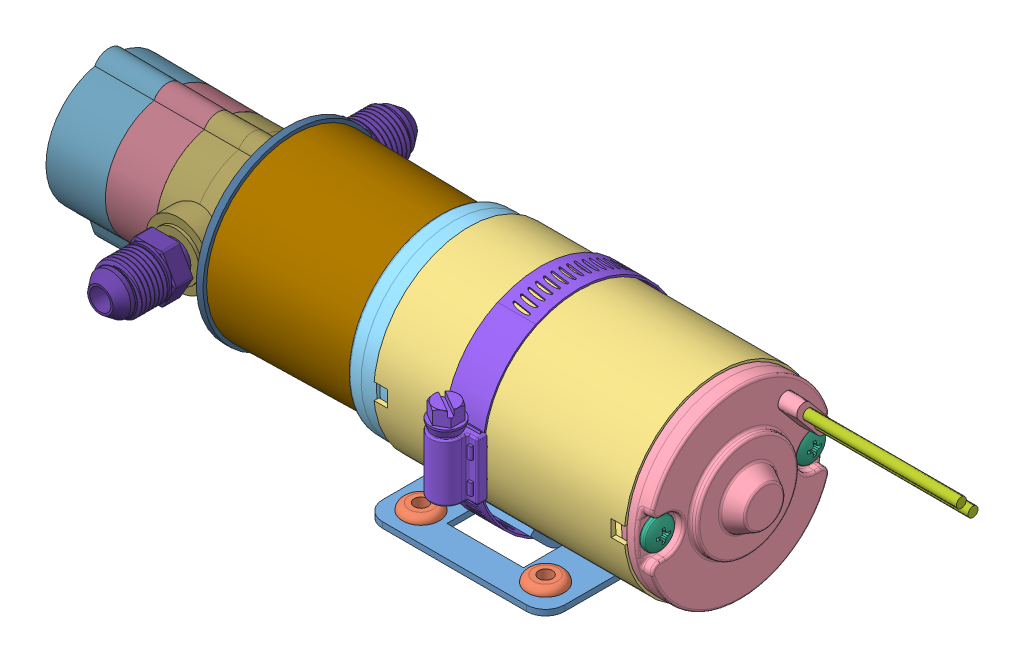
SolidWorks assembly P-SERIES, configuration Default. Lengths in mm.
Overall size (266.07 68.69 100.84).
26 component instances, 17 part files, 51 mates.
Components (placement in the parent):
- BAND CLAMP MOUNTING PLATE^P-SERIES-1: BAND CLAMP MOUNTING PLATE^P-SERIES [Default] at origin size (60.32 13.25 69.85) (virtual)
  - BAND CLAMP MOUNTING PLATE^BAND CLAMP MOUNTING PLATE_P-SERIES-1: BAND CLAMP MOUNTING PLATE^BAND CLAMP MOUNTING PLATE_P-SERIES [01] at (0 1.905 0) x (0 0 1) z (0 -1 0) size (69.85 60.32 11.06) (virtual)
  - GROMMET^BAND CLAMP MOUNTING PLATE_P-SERIES-1: GROMMET^BAND CLAMP MOUNTING PLATE_P-SERIES [01] at (20.6375 1.016 -25.4) size (12.19 6.4 12.19) (virtual)
  - GROMMET^BAND CLAMP MOUNTING PLATE_P-SERIES-2: GROMMET^BAND CLAMP MOUNTING PLATE_P-SERIES [01] at (-20.6375 1.016 -25.4) size (12.19 6.4 12.19) (virtual)
  - GROMMET^BAND CLAMP MOUNTING PLATE_P-SERIES-3: GROMMET^BAND CLAMP MOUNTING PLATE_P-SERIES [01] at (20.6375 1.016 25.4) size (12.19 6.4 12.19) (virtual)
  - GROMMET^BAND CLAMP MOUNTING PLATE_P-SERIES-4: GROMMET^BAND CLAMP MOUNTING PLATE_P-SERIES [01] at (-20.6375 1.016 25.4) size (12.19 6.4 12.19) (virtual)
- 12VDC MOTOR^P-SERIES-1: 12VDC MOTOR^P-SERIES [Default] at (11.3375 34.421 0) size (156.2 63 63) (virtual)
  - 12VDC MOTOR HOUSING^12VDC MOTOR_P-SERIES-1: 12VDC MOTOR HOUSING^12VDC MOTOR_P-SERIES [01] at origin size (83 63 63) (virtual)
  - SOURCE END CASTING^12VDC MOTOR_P-SERIES-1: SOURCE END CASTING^12VDC MOTOR_P-SERIES [01] at origin size (18.93 61.6 61.6) (virtual)
  - COUPLER END CASTING^12VDC MOTOR_P-SERIES-1: COUPLER END CASTING^12VDC MOTOR_P-SERIES [01] at origin size (12.31 61.6 61.6) (virtual)
  - PHIL MACHINE SCREW^12VDC MOTOR_P-SERIES-1: PHIL MACHINE SCREW^12VDC MOTOR_P-SERIES [93802A733] at (28.998 0 25) x (0 1 0) z (1 0 0) size (10.35 10.24 95.59) (virtual)
  - PHIL MACHINE SCREW^12VDC MOTOR_P-SERIES-2: PHIL MACHINE SCREW^12VDC MOTOR_P-SERIES [93802A733] at (28.998 0 -25) x (0 1 0) z (1 0 0) size (10.35 10.24 95.59) (virtual)
  - WIRES^12VDC MOTOR_P-SERIES-1: WIRES^12VDC MOTOR_P-SERIES [01] at (54.5 0 0) x (0 0 -1) z (1 0 0) size (7.16 7.9 57.15) (virtual)
- WORM-DRIVE CLAMP^P-SERIES-1: WORM-DRIVE CLAMP^P-SERIES [01] at (0 32.5835 0) x (0 1 0) z (1 0 0) size (67.85 76.82 17.02) (virtual)
- COUPLER^P-SERIES-1: COUPLER^P-SERIES [01] at (-63.8125 34.421 0) size (48.5 58 58) (virtual)
- COUPLER PLATE^P-SERIES-1: COUPLER PLATE^P-SERIES [01] at (-88.0625 34.421 0) x (0 0 1) z (-1 0 0) size (60.3 60.3 2.25) (virtual)
- Socket Head Screw^P-SERIES-1: Socket Head Screw^P-SERIES [01] at (-91.8125 59.671 0) size (61.5 4.5 4.5) (virtual)
- Socket Head Screw^P-SERIES-2: Socket Head Screw^P-SERIES [01] at (-91.8125 18.6779 -19.7412) x (1 0 0) z (0 0 -1) size (61.5 4.5 4.5) (virtual)
- Socket Head Screw^P-SERIES-3: Socket Head Screw^P-SERIES [01] at (-91.8125 18.6779 19.7412) size (61.5 4.5 4.5) (virtual)
- PUMP01^P-SERIES-1: PUMP01^P-SERIES [01] at (-90.3125 34.421 0) x (0 0 1) z (-1 0 0) size (51.25 53.2 23.06) (virtual)
- PUMP02^P-SERIES-1: PUMP02^P-SERIES [01] at (-113.3725 34.421 0) x (0 0 1) z (-1 0 0) size (41.29 53.29 16.56) (virtual)
- PUMP03^P-SERIES-1: PUMP03^P-SERIES [01] at (-129.9325 34.421 0) x (0 0 1) z (-1 0 0) size (41.63 53.63 19.5) (virtual)
- STUDS^P-SERIES-1: STUDS^P-SERIES [01] at (-149.4325 34.421 0) x (0 0 1) z (-1 0 0) size (3.17 46.18 59.12) (virtual)
- NUTS^P-SERIES-1: NUTS^P-SERIES [01] at (-144.67 34.421 0) x (0 0 1) z (-1 0 0) size (5.84 48.84 4.32) (virtual)
- .625-18 37°JIC X .125MNPT STRAIGHT FITTING^P-SERIES-1: .625-18 37°JIC X .125MNPT STRAIGHT FITTING^P-SERIES [01] at (-101.8425 34.421 -28.575) x (0 0 1) z (-1 0 0) size (35.26 16.42 18.33) (virtual)
- .625-18 37°JIC X .125MNPT STRAIGHT FITTING^P-SERIES-2: .625-18 37°JIC X .125MNPT STRAIGHT FITTING^P-SERIES [01] at (-101.8425 34.3048 28.575) x (0 0 -1) z (-1 0 0) size (35.26 16.42 18.33) (virtual)
Mates (geometry in assembly coordinates):
- Coincident9: coincident: plane of BAND CLAMP MOUNTING PLATE^P-SERIES-1/BAND CLAMP MOUNTING PLATE^BAND CLAMP MOUNTING PLATE_P-SERIES-1 through (0 1.905 0) normal (-1 0 0); plane of assembly through (0 0 0) normal (1 0 0)
- Coincident10: coincident: plane of BAND CLAMP MOUNTING PLATE^P-SERIES-1/BAND CLAMP MOUNTING PLATE^BAND CLAMP MOUNTING PLATE_P-SERIES-1 through (0 1.905 0) normal (0 0 1); plane of assembly through (0 0 0) normal (0 0 1)
- Coincident11: coincident: plane of BAND CLAMP MOUNTING PLATE^P-SERIES-1/BAND CLAMP MOUNTING PLATE^BAND CLAMP MOUNTING PLATE_P-SERIES-1 through (23.8125 0 -28.575) normal (0 -1 0); plane of assembly through (0 0 0) normal (0 1 0)
- Parallel5: parallel: plane of BAND CLAMP MOUNTING PLATE^P-SERIES-1/GROMMET^BAND CLAMP MOUNTING PLATE_P-SERIES-1 through (20.6375 1.016 -25.4) normal (0 0 1); plane of assembly through (0 0 0) normal (0 0 1)
- Parallel6: parallel: plane of BAND CLAMP MOUNTING PLATE^P-SERIES-1/GROMMET^BAND CLAMP MOUNTING PLATE_P-SERIES-2 through (-20.6375 1.016 -25.4) normal (0 0 1); plane of assembly through (0 0 0) normal (0 0 1)
- Concentric5: concentric: circle of BAND CLAMP MOUNTING PLATE^P-SERIES-1/BAND CLAMP MOUNTING PLATE^BAND CLAMP MOUNTING PLATE_P-SERIES-1; cylinder of 12VDC MOTOR^P-SERIES-1/12VDC MOTOR HOUSING^12VDC MOTOR_P-SERIES-1 through (52.8375 34.421 0) axis (-1 0 0) radius 31.5
- Parallel7: parallel: plane of ? through (11.3375 34.421 0) normal (0 0 1); plane of assembly through (0 0 0) normal (0 0 1)
- Coincident12: coincident: plane of BAND CLAMP MOUNTING PLATE^P-SERIES-1/BAND CLAMP MOUNTING PLATE^BAND CLAMP MOUNTING PLATE_P-SERIES-1 through (-30.1625 0 -28.575) normal (-1 0 0); plane of 12VDC MOTOR^P-SERIES-1/12VDC MOTOR HOUSING^12VDC MOTOR_P-SERIES-1 through (-30.1625 34.421 0) normal (-1 0 0)
- Coincident13: coincident: plane of BAND CLAMP MOUNTING PLATE^P-SERIES-1 through (0 0 0) normal (1 0 0); plane of WORM-DRIVE CLAMP^P-SERIES-1 through (0 32.5835 0) normal (1 0 0)
- Parallel8: parallel: plane of BAND CLAMP MOUNTING PLATE^P-SERIES-1/BAND CLAMP MOUNTING PLATE^BAND CLAMP MOUNTING PLATE_P-SERIES-1 through (23.8125 1.905 -28.575) normal (0 1 0); plane of WORM-DRIVE CLAMP^P-SERIES-1 through (0 49.9419 42.3027) normal (0 1 0)
- Coincident14: coincident: plane of WORM-DRIVE CLAMP^P-SERIES-1 through (0 32.5835 0) normal (0 0 1); plane of assembly through (0 0 0) normal (0 0 1)
- Tangent1: tangent: cylinder of 12VDC MOTOR^P-SERIES-1/12VDC MOTOR HOUSING^12VDC MOTOR_P-SERIES-1 through (52.8375 34.421 0) axis (-1 0 0) radius 31.5; cylinder of WORM-DRIVE CLAMP^P-SERIES-1 through (6.35 32.5835 0) axis (-1 0 0) radius 33.3375
- Coincident15: coincident: plane of 12VDC MOTOR^P-SERIES-1/COUPLER END CASTING^12VDC MOTOR_P-SERIES-1 through (-39.5625 65.0639 0) normal (-1 0 0); plane of COUPLER^P-SERIES-1 through (-39.5625 53.0494 0) normal (1 0 0)
- Coincident16: coincident: plane of COUPLER^P-SERIES-1 through (-63.8125 34.421 0) normal (0 0 1); plane of assembly through (0 0 0) normal (0 0 1)
- Concentric6: concentric: cylinder of 12VDC MOTOR^P-SERIES-1/12VDC MOTOR HOUSING^12VDC MOTOR_P-SERIES-1 through (52.8375 34.421 0) axis (-1 0 0) radius 31.5; cylinder of COUPLER^P-SERIES-1 through (-88.0625 34.421 0) axis (-1 0 0) radius 18.6284
- InPlace1: in place: plane of ? through (-88.0625 63.071 0) normal (-1 0 0); plane of ? through (-88.0625 0 0) normal (-1 0 0); moOrthogonalPlaneRef_w of ? through (-88.0625 63.071 0) normal (-1 0 0); plane of ? through (-88.0625 0 0) normal (0 1 0); plane of ? through (-88.0625 63.071 0) normal (-1 0 0); plane of ? through (-88.0625 0 0) normal (0 0 1); plane of COUPLER^P-SERIES-1 through (-88.0625 63.421 0) normal (-1 0 0); unknown of COUPLER PLATE^P-SERIES-1
- Coincident17: coincident: plane of COUPLER^P-SERIES-1; plane of COUPLER PLATE^P-SERIES-1
- Coincident18: coincident: moOrthogonalPlaneRef_w of COUPLER^P-SERIES-1 through (-88.0625 34.421 0) normal (0 1 0); plane of COUPLER PLATE^P-SERIES-1 through (-88.0625 34.421 0) normal (0 1 0)
- Coincident19: coincident: moOrthogonalPlaneRef_w of COUPLER^P-SERIES-1 through (-88.0625 34.421 0) normal (0 0 -1); plane of COUPLER PLATE^P-SERIES-1 through (-88.0625 34.421 0) normal (0 0 1)
- InPlace2: in place: plane of ? through (-90.3125 34.671 0) normal (-1 0 0); plane of ? through (-90.3125 0 0) normal (-1 0 0); plane of ? through (-90.3125 34.671 0) normal (-1 0 0); plane of ? through (-90.3125 0 0) normal (0 1 0); plane of ? through (-90.3125 34.671 0) normal (-1 0 0); plane of ? through (-90.3125 0 0) normal (0 0 1); plane of COUPLER PLATE^P-SERIES-1 through (-90.3125 34.421 0) normal (-1 0 0); unknown of PUMP01^P-SERIES-1
- Coincident20: coincident: plane of COUPLER PLATE^P-SERIES-1; plane of PUMP01^P-SERIES-1
- Coincident21: coincident: moOrthogonalPlaneRef_w of COUPLER PLATE^P-SERIES-1 through (-90.3125 34.421 0) normal (0 1 0); plane of PUMP01^P-SERIES-1 through (-90.3125 34.421 0) normal (0 1 0)
- Coincident22: coincident: moOrthogonalPlaneRef_w of COUPLER PLATE^P-SERIES-1 through (-90.3125 34.421 0) normal (0 0 -1); plane of PUMP01^P-SERIES-1 through (-90.3125 34.421 0) normal (0 0 1)
- InPlace3: in place: plane of ? through (-113.3725 34.671 0) normal (-1 0 0); plane of ? through (-113.3725 0 0) normal (-1 0 0); plane of ? through (-113.3725 34.671 0) normal (-1 0 0); plane of ? through (-113.3725 0 0) normal (0 1 0); plane of ? through (-113.3725 34.671 0) normal (-1 0 0); plane of ? through (-113.3725 0 0) normal (0 0 1); plane of PUMP01^P-SERIES-1 through (-113.3725 34.421 0) normal (-1 0 0); unknown of PUMP02^P-SERIES-1
- Coincident23: coincident: plane of PUMP01^P-SERIES-1; plane of PUMP02^P-SERIES-1
- Coincident24: coincident: moOrthogonalPlaneRef_w of PUMP01^P-SERIES-1 through (-113.3725 34.421 0) normal (0 1 0); plane of PUMP02^P-SERIES-1 through (-113.3725 34.421 0) normal (0 1 0)
- Coincident25: coincident: moOrthogonalPlaneRef_w of PUMP01^P-SERIES-1 through (-113.3725 34.421 0) normal (0 0 -1); plane of PUMP02^P-SERIES-1 through (-113.3725 34.421 0) normal (0 0 1)
- InPlace4: in place: plane of ? through (-129.9325 9.221 0) normal (-1 0 0); plane of ? through (-129.9325 0 0) normal (-1 0 0); plane of ? through (-129.9325 9.221 0) normal (-1 0 0); plane of ? through (-129.9325 0 0) normal (0 1 0); plane of ? through (-129.9325 9.221 0) normal (-1 0 0); plane of ? through (-129.9325 0 0) normal (0 0 1); plane of PUMP02^P-SERIES-1 through (-129.9325 9.171 0) normal (-1 0 0); unknown of PUMP03^P-SERIES-1
- Coincident26: coincident: plane of PUMP02^P-SERIES-1; plane of PUMP03^P-SERIES-1
- Coincident27: coincident: moOrthogonalPlaneRef_w of PUMP02^P-SERIES-1 through (-129.9325 34.421 0) normal (0 1 0); plane of PUMP03^P-SERIES-1 through (-129.9325 34.421 0) normal (0 1 0)
- Coincident28: coincident: moOrthogonalPlaneRef_w of PUMP02^P-SERIES-1 through (-129.9325 34.421 0) normal (0 0 -1); plane of PUMP03^P-SERIES-1 through (-129.9325 34.421 0) normal (0 0 1)
- InPlace5: in place: plane of ? through (-149.4325 9.221 0) normal (-1 0 0); plane of ? through (-149.4325 0 0) normal (-1 0 0); plane of ? through (-149.4325 9.221 0) normal (-1 0 0); plane of ? through (-149.4325 0 0) normal (0 1 0); plane of ? through (-149.4325 9.221 0) normal (-1 0 0); plane of ? through (-149.4325 0 0) normal (0 0 1); plane of PUMP03^P-SERIES-1 through (-149.4325 9.171 0) normal (-1 0 0); unknown of STUDS^P-SERIES-1
- Coincident29: coincident: plane of PUMP03^P-SERIES-1; plane of STUDS^P-SERIES-1
- Coincident30: coincident: moOrthogonalPlaneRef_w of PUMP03^P-SERIES-1 through (-149.4325 34.421 0) normal (0 1 0); plane of STUDS^P-SERIES-1 through (-149.4325 34.421 0) normal (0 1 0)
- Coincident31: coincident: moOrthogonalPlaneRef_w of PUMP03^P-SERIES-1 through (-149.4325 34.421 0) normal (0 0 -1); plane of STUDS^P-SERIES-1 through (-149.4325 34.421 0) normal (0 0 1)
- InPlace6: in place: plane of ? through (-144.67 52.221 1.9844) normal (-1 0 0); plane of ? through (-144.67 0 0) normal (-1 0 0); plane of ? through (-144.67 52.221 1.9844) normal (-1 0 0); plane of ? through (-144.67 0 0) normal (0 1 0); plane of ? through (-144.67 52.221 1.9844) normal (-1 0 0); plane of ? through (-144.67 0 0) normal (0 0 1); plane of PUMP03^P-SERIES-1 through (-144.67 52.171 1.9844) normal (-1 0 0); unknown of NUTS^P-SERIES-1
- Coincident32: coincident: plane of PUMP03^P-SERIES-1; plane of NUTS^P-SERIES-1
- Coincident33: coincident: moOrthogonalPlaneRef_w of PUMP03^P-SERIES-1 through (-144.67 34.421 0) normal (0 1 0); plane of NUTS^P-SERIES-1 through (-144.67 34.421 0) normal (0 1 0)
- Coincident34: coincident: moOrthogonalPlaneRef_w of PUMP03^P-SERIES-1 through (-144.67 34.421 0) normal (0 0 -1); plane of NUTS^P-SERIES-1 through (-144.67 34.421 0) normal (0 0 1)
- Coincident38: coincident: plane of COUPLER PLATE^P-SERIES-1 through (-90.3125 34.421 0) normal (-1 0 0); circle of Socket Head Screw^P-SERIES-1
- Concentric10: concentric: circle of COUPLER PLATE^P-SERIES-1; cylinder of Socket Head Screw^P-SERIES-1 through (-123.5625 59.671 0) axis (-1 0 0) radius 2.25
- Parallel9: parallel: plane of Socket Head Screw^P-SERIES-1 through (-91.8125 59.671 0) normal (0 0 1); plane of assembly through (0 0 0) normal (0 0 1)
- Concentric11: concentric: cylinder of COUPLER^P-SERIES-1 through (-39.5625 18.6779 -19.7412) axis (-1 0 0) radius 1.5; cylinder of Socket Head Screw^P-SERIES-2 through (-123.5625 18.6779 -19.7412) axis (-1 0 0) radius 2.25
- Coincident40: coincident: plane of COUPLER PLATE^P-SERIES-1 through (-90.3125 34.421 0) normal (-1 0 0); plane of Socket Head Screw^P-SERIES-2 through (-90.3125 16.4279 -19.7412) normal (1 0 0)
- Concentric12: concentric: cylinder of COUPLER^P-SERIES-1 through (-39.5625 18.6779 19.7412) axis (-1 0 0) radius 1.5; cylinder of Socket Head Screw^P-SERIES-3 through (-123.5625 18.6779 19.7412) axis (-1 0 0) radius 1.25
- Coincident41: coincident: plane of Socket Head Screw^P-SERIES-1 through (-91.8125 59.671 0) normal (-1 0 0); plane of Socket Head Screw^P-SERIES-3 through (-91.8125 18.6779 19.7412) normal (-1 0 0)
- Parallel10: parallel: plane of Socket Head Screw^P-SERIES-2 through (-91.8125 18.6779 -19.7412) normal (0 0 -1); plane of assembly through (0 0 0) normal (0 0 1)
- Parallel11: parallel: plane of Socket Head Screw^P-SERIES-3 through (-91.8125 18.6779 19.7412) normal (0 0 1); plane of assembly through (0 0 0) normal (0 0 1)
- Concentric13: concentric: circle of PUMP01^P-SERIES-1; cylinder of .625-18 37°JIC X .125MNPT STRAIGHT FITTING^P-SERIES-1 through (-101.8425 34.421 -50.419) axis (0 0 -1) radius 3.5052
- Distance1: distance = 50.419 mm: plane of .625-18 37°JIC X .125MNPT STRAIGHT FITTING^P-SERIES-1 through (-97.6515 34.421 -50.419) normal (0 0 -1); plane of assembly through (0 0 0) normal (0 0 1)
- Parallel12: parallel: plane of .625-18 37°JIC X .125MNPT STRAIGHT FITTING^P-SERIES-1 through (-101.8425 34.421 -28.575) normal (-1 0 0); plane of assembly through (0 0 0) normal (1 0 0)
